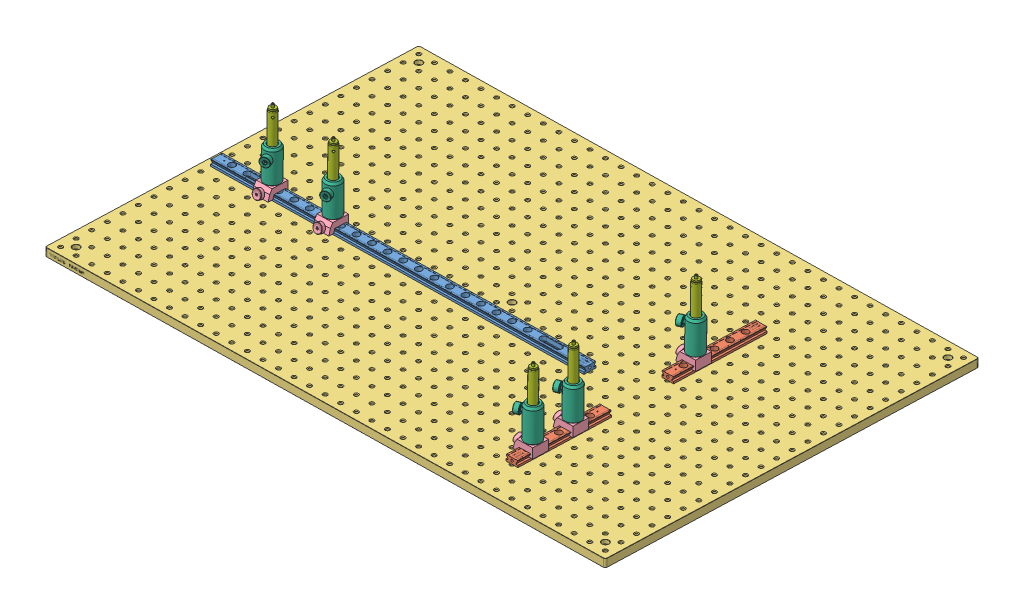
SolidWorks assembly OpenCALAssembly, configuration Default. Lengths in mm.
Overall size (900.56 165.28 600.29).
29 component instances, 7 part files, 30 mates.
Components (placement in the parent):
- RLA600_M-Solidworks-1: RLA600_M-Solidworks [Default] at (212.74 428.5429 890.6377) x (0.000793 -0.03295 -0.999457) z (0.999847 0.01748 0.000217) size (19.05 9.53 600)
- RLA150_M-Solidworks-1: RLA150_M-Solidworks [Default] at (587.7819 430.9791 765.7872) x (0.999847 0.01748 0.000217) z (-0.000793 0.03295 0.999457) size (19.05 9.53 150)
- RLA150_M-Solidworks-2: RLA150_M-Solidworks [Default] at (587.5835 439.2167 1015.6513) x (-0.999847 -0.01748 -0.000217) z (0.000793 -0.03295 -0.999457) size (19.05 9.53 150)
- MB6090_M-Solidworks-1: MB6090_M-Solidworks [Default] at (350.5593 411.9431 853.774) x (0.999847 0.01748 0.000217) z (-0.000793 0.03295 0.999457) size (900 12.7 600)
- Rail-Post^OpenCALAssembly-1: Rail-Post^OpenCALAssembly [Default] at (243.8757 -121.8493 -138.0671) x (0.999969 -0.007878 0.000659) z (-0.000645 0.001893 0.999998) size (37.63 121.62 44.58) (virtual)
  - RC1-Solidworks-1: RC1-Solidworks [Default] at (-258.0543 541.4605 1048.8284) x (0.999678 0.025357 -0.000394) z (-0.000279 0.026514 0.999648) size (25.4 16.53 39.23)
  - socket head cap screw_am-1: socket head cap screw_am [B18.3.1M - 6 x 1.0 x 10 Hex SHCS -- 10NHX] at (-245.5045 547.2464 1029.7741) x (-0.025359 0.999327 -0.026513) z (0.026513 0.027184 0.999279) size (16 10 10)
  - PH50_M-Solidworks-1: PH50_M-Solidworks [Default] at (-244.0284 576.1062 1033.7923) x (0.926646 0.013547 -0.375692) z (0.37508 0.034095 0.926365) size (25 50.44 35.14)
  - TR75_M-Solidworks-1: TR75_M-Solidworks [Default] at (-246.3606 580.9852 1028.879) x (0.691707 -0.001607 -0.722176) z (0.721732 0.036653 0.691201) size (12.67 80.02 12.87)
- Rail-Post^OpenCALAssembly-2: Rail-Post^OpenCALAssembly [Default] at (341.3904 -120.1445 -138.0459) x (0.999969 -0.007878 0.000659) z (-0.000645 0.001893 0.999998) size (37.63 121.62 44.58) (virtual)
  - RC1-Solidworks-1: RC1-Solidworks [Default] at (-258.0543 541.4605 1048.8284) x (0.999678 0.025357 -0.000394) z (-0.000279 0.026514 0.999648) size (25.4 16.53 39.23)
  - socket head cap screw_am-1: socket head cap screw_am [B18.3.1M - 6 x 1.0 x 10 Hex SHCS -- 10NHX] at (-245.5045 547.2464 1029.7741) x (-0.025359 0.999327 -0.026513) z (0.026513 0.027184 0.999279) size (16 10 10)
  - PH50_M-Solidworks-1: PH50_M-Solidworks [Default] at (-244.0284 576.1062 1033.7923) x (0.926646 0.013547 -0.375692) z (0.37508 0.034095 0.926365) size (25 50.44 35.14)
  - TR75_M-Solidworks-1: TR75_M-Solidworks [Default] at (-246.3606 580.9852 1028.879) x (0.691707 -0.001607 -0.722176) z (0.721732 0.036653 0.691201) size (12.67 80.02 12.87)
- Rail-Post^OpenCALAssembly-4: Rail-Post^OpenCALAssembly [Default] at (1642.5862 -51.8881 1242.018) x (0.000044 0.007607 0.999971) z (-0.998822 -0.048519 0.000413) size (37.63 121.62 44.58) (virtual)
  - RC1-Solidworks-1: RC1-Solidworks [Default] at (-258.0543 541.4605 1048.8284) x (0.999678 0.025357 -0.000394) z (-0.000279 0.026514 0.999648) size (25.4 16.53 39.23)
  - socket head cap screw_am-1: socket head cap screw_am [B18.3.1M - 6 x 1.0 x 10 Hex SHCS -- 10NHX] at (-245.5045 547.2464 1029.7741) x (-0.025359 0.999327 -0.026513) z (0.026513 0.027184 0.999279) size (16 10 10)
  - PH50_M-Solidworks-1: PH50_M-Solidworks [Default] at (-244.0284 576.1062 1033.7923) x (0.926646 0.013547 -0.375692) z (0.37508 0.034095 0.926365) size (25 50.44 35.14)
  - TR75_M-Solidworks-1: TR75_M-Solidworks [Default] at (-246.3606 580.9852 1028.879) x (0.691707 -0.001607 -0.722176) z (0.721732 0.036653 0.691201) size (12.67 80.02 12.87)
- Rail-Post^OpenCALAssembly-6: Rail-Post^OpenCALAssembly [Default] at (1642.7424 -58.374 1045.2874) x (0.000044 0.007607 0.999971) z (-0.998822 -0.048519 0.000413) size (37.63 121.62 44.58) (virtual)
  - RC1-Solidworks-1: RC1-Solidworks [Default] at (-258.0543 541.4605 1048.8284) x (0.999678 0.025357 -0.000394) z (-0.000279 0.026514 0.999648) size (25.4 16.53 39.23)
  - socket head cap screw_am-1: socket head cap screw_am [B18.3.1M - 6 x 1.0 x 10 Hex SHCS -- 10NHX] at (-245.5045 547.2464 1029.7741) x (-0.025359 0.999327 -0.026513) z (0.026513 0.027184 0.999279) size (16 10 10)
  - PH50_M-Solidworks-1: PH50_M-Solidworks [Default] at (-244.0284 576.1062 1033.7923) x (0.926646 0.013547 -0.375692) z (0.37508 0.034095 0.926365) size (25 50.44 35.14)
  - TR75_M-Solidworks-1: TR75_M-Solidworks [Default] at (-246.3606 580.9852 1028.879) x (0.691707 -0.001607 -0.722176) z (0.721732 0.036653 0.691201) size (12.67 80.02 12.87)
- Rail-Post^OpenCALAssembly-8: Rail-Post^OpenCALAssembly [Default] at (1642.581 -49.6743 1306.6232) x (0.000044 0.007607 0.999971) z (-0.998822 -0.048519 0.000413) size (37.63 121.62 44.58) (virtual)
  - RC1-Solidworks-1: RC1-Solidworks [Default] at (-258.0543 541.4605 1048.8284) x (0.999678 0.025357 -0.000394) z (-0.000279 0.026514 0.999648) size (25.4 16.53 39.23)
  - socket head cap screw_am-1: socket head cap screw_am [B18.3.1M - 6 x 1.0 x 10 Hex SHCS -- 10NHX] at (-245.5045 547.2464 1029.7741) x (-0.025359 0.999327 -0.026513) z (0.026513 0.027184 0.999279) size (16 10 10)
  - PH50_M-Solidworks-1: PH50_M-Solidworks [Default] at (-244.0284 576.1062 1033.7923) x (0.926646 0.013547 -0.375692) z (0.37508 0.034095 0.926365) size (25 50.44 35.14)
  - TR75_M-Solidworks-1: TR75_M-Solidworks [Default] at (-246.3606 580.9852 1028.879) x (0.691707 -0.001607 -0.722176) z (0.721732 0.036653 0.691201) size (12.67 80.02 12.87)
Mates (geometry in assembly coordinates):
- Concentric5: concentric aligned: cylinder of RLA600_M-Solidworks-1 through (-62.2911 427.9239 890.4398) axis (-0.017463 0.999304 -0.032959) radius 3.3655; circle of MB6090_M-Solidworks-1
- Concentric6: concentric aligned: cylinder of RLA600_M-Solidworks-1 through (487.6248 437.538 890.5594) axis (-0.017463 0.999304 -0.032959) radius 3.3655; circle of MB6090_M-Solidworks-1
- Coincident8: coincident anti-aligned: plane of RLA600_M-Solidworks-1 through (512.7753 429.0243 900.3902) normal (0.017463 -0.999304 0.032959); plane of MB6090_M-Solidworks-1 through (-96.8299 426.6069 1150.0969) normal (-0.017463 0.999304 -0.032959)
- Coincident9: coincident anti-aligned: plane of RLA150_M-Solidworks-2 through (578.2082 431.5024 940.8575) normal (0.017463 -0.999304 0.032959); plane of MB6090_M-Solidworks-1 through (-96.8299 426.6069 1150.0969) normal (-0.017463 0.999304 -0.032959)
- Coincident10: coincident anti-aligned: plane of RLA150_M-Solidworks-1 through (597.3346 428.5404 840.9159) normal (0.017463 -0.999304 0.032959); plane of MB6090_M-Solidworks-1 through (-96.8299 426.6069 1150.0969) normal (-0.017463 0.999304 -0.032959)
- Concentric7: concentric aligned: cylinder of RLA600_M-Solidworks-1 through (-12.2988 428.7979 890.4507) axis (-0.017463 0.999304 -0.032959) radius 5.1562; cylinder of socket head cap screw_am-2 through (-200.2466 470.3352 1027.7075) axis (-0.025357 0.999196 -0.031056) radius 5
- Parallel5: parallel aligned: plane of RLA600_M-Solidworks-1 through (-87.2867 427.5323 884.1048) normal (-0.999847 -0.01748 -0.000217); plane of Rail-Post^OpenCALAssembly-1/RC1-Solidworks-1 through (-10.5574 422.7142 877.982) normal (-0.999847 -0.01748 -0.000217)
- Coincident23: coincident anti-aligned: plane of RLA600_M-Solidworks-1 through (512.6371 437.1668 881.4679) normal (0.009352 -0.524324 -0.851468); plane of Rail-Post^OpenCALAssembly-1/RC1-Solidworks-1 through (14.7938 425.6602 883.0857) normal (-0.009352 0.524324 0.851468)
- Parallel6: parallel aligned: plane of RLA600_M-Solidworks-1 through (-87.2867 427.5323 884.1048) normal (-0.999847 -0.01748 -0.000217); plane of Rail-Post^OpenCALAssembly-1/RC1-Solidworks-1 through (-10.5574 422.7142 877.982) normal (-0.999847 -0.01748 -0.000217)
- Coincident24: coincident: line of RLA600_M-Solidworks-1 through (512.6238 437.9283 881.4428) axis (-0.999847 -0.01748 -0.000217); plane of Rail-Post^OpenCALAssembly-1/RC1-Solidworks-1 through (14.7185 429.7567 900.0847) normal (0.017467 -0.999444 0.028416)
- Parallel7: parallel aligned: plane of RLA600_M-Solidworks-1 through (-87.2867 427.5323 884.1048) normal (-0.999847 -0.01748 -0.000217); plane of Rail-Post^OpenCALAssembly-2/RC1-Solidworks-1 through (86.9572 424.419 878.0032) normal (-0.999847 -0.01748 -0.000217)
- Coincident25: coincident anti-aligned: plane of RLA600_M-Solidworks-1 through (512.6371 437.1668 881.4679) normal (0.009352 -0.524324 -0.851468); plane of Rail-Post^OpenCALAssembly-2/RC1-Solidworks-1 through (112.3085 427.365 883.1069) normal (-0.009352 0.524324 0.851468)
- Parallel8: parallel aligned: plane of RLA600_M-Solidworks-1 through (-87.2867 427.5323 884.1048) normal (-0.999847 -0.01748 -0.000217); plane of Rail-Post^OpenCALAssembly-2/RC1-Solidworks-1 through (86.9572 424.419 878.0032) normal (-0.999847 -0.01748 -0.000217)
- Coincident26: coincident: line of RLA600_M-Solidworks-1 through (512.6238 437.9283 881.4428) axis (-0.999847 -0.01748 -0.000217); plane of Rail-Post^OpenCALAssembly-2/RC1-Solidworks-1 through (112.2332 431.4615 900.1059) normal (0.017467 -0.999444 0.028416)
- Parallel11: parallel aligned: plane of RLA150_M-Solidworks-2 through (581.2418 441.0767 940.5442) normal (0.000793 -0.03295 -0.999457); plane of Rail-Post^OpenCALAssembly-4/RC1-Solidworks-1 through (600.2998 436.7637 980.2933) normal (0.000793 -0.03295 -0.999457)
- Coincident29: coincident anti-aligned: plane of RLA150_M-Solidworks-2 through (596.6959 440.5852 940.5727) normal (0.876819 -0.480535 0.016538); plane of Rail-Post^OpenCALAssembly-4/RC1-Solidworks-1 through (595.0618 439.8415 1005.6015) normal (-0.876819 0.480535 -0.016538)
- Parallel12: parallel aligned: plane of RLA150_M-Solidworks-2 through (581.2418 441.0767 940.5442) normal (0.000793 -0.03295 -0.999457); plane of Rail-Post^OpenCALAssembly-4/RC1-Solidworks-1 through (600.2998 436.7637 980.2933) normal (0.000793 -0.03295 -0.999457)
- Coincident30: coincident: line of RLA150_M-Solidworks-2 through (596.6826 441.3467 940.5476) axis (-0.000793 0.03295 0.999457); plane of Rail-Post^OpenCALAssembly-4/RC1-Solidworks-1 through (577.8779 443.0744 1005.4813) normal (0.022008 -0.999214 0.03296)
- Concentric13: concentric anti-aligned: cylinder of RLA150_M-Solidworks-2 through (587.55 441.7572 965.5404) axis (-0.017463 0.999304 -0.032959) radius 5.1562; cone of MB6090_M-Solidworks-1 through (587.7119 432.4927 965.8459) axis (0.017463 -0.999304 0.032959)
- Concentric14: concentric anti-aligned: cylinder of RLA150_M-Solidworks-2 through (587.4707 445.0522 1065.4861) axis (-0.017463 0.999304 -0.032959) radius 5.1562; cone of MB6090_M-Solidworks-1 through (587.6326 435.7877 1065.7916) axis (0.017463 -0.999304 0.032959)
- Concentric15: concentric anti-aligned: cylinder of RLA150_M-Solidworks-1 through (587.669 436.8147 815.6219) axis (-0.017463 0.999304 -0.032959) radius 3.3655; cone of MB6090_M-Solidworks-1 through (587.8309 427.5501 815.9274) axis (0.017463 -0.999304 0.032959)
- Concentric16: concentric anti-aligned: cylinder of RLA150_M-Solidworks-1 through (587.7484 433.5197 715.6762) axis (-0.017463 0.999304 -0.032959) radius 5.1562; cone of MB6090_M-Solidworks-1 through (587.9103 424.2551 715.9818) axis (0.017463 -0.999304 0.032959)
- Parallel13: parallel aligned: plane of RLA150_M-Solidworks-2 through (581.2418 441.0767 940.5442) normal (0.000793 -0.03295 -0.999457); plane of Rail-Post^OpenCALAssembly-6/RC1-Solidworks-1 through (600.456 430.2779 783.5628) normal (0.000793 -0.03295 -0.999457)
- Coincident31: coincident anti-aligned: plane of RLA150_M-Solidworks-2 through (596.6959 440.5852 940.5727) normal (0.876819 -0.480535 0.016538); plane of Rail-Post^OpenCALAssembly-6/RC1-Solidworks-1 through (595.218 433.3557 808.8709) normal (-0.876819 0.480535 -0.016538)
- Parallel14: parallel aligned: plane of RLA150_M-Solidworks-2 through (581.2418 441.0767 940.5442) normal (0.000793 -0.03295 -0.999457); plane of Rail-Post^OpenCALAssembly-6/RC1-Solidworks-1 through (600.456 430.2779 783.5628) normal (0.000793 -0.03295 -0.999457)
- Coincident32: coincident: line of RLA150_M-Solidworks-2 through (596.6826 441.3467 940.5476) axis (-0.000793 0.03295 0.999457); plane of Rail-Post^OpenCALAssembly-6/RC1-Solidworks-1 through (578.0341 436.5886 808.7507) normal (0.022008 -0.999214 0.03296)
- Parallel17: parallel anti-aligned: plane of RLA150_M-Solidworks-1 through (593.9684 438.0028 840.6013) normal (-0.000793 0.03295 0.999457); plane of Rail-Post^OpenCALAssembly-8/RC1-Solidworks-1 through (600.2946 438.9776 1044.8985) normal (0.000793 -0.03295 -0.999457)
- Coincident35: coincident anti-aligned: plane of RLA150_M-Solidworks-1 through (596.7753 437.2902 840.627) normal (0.876819 -0.480535 0.016538); plane of Rail-Post^OpenCALAssembly-8/RC1-Solidworks-1 through (595.0565 442.0554 1070.2067) normal (-0.876819 0.480535 -0.016538)
- Parallel18: parallel aligned: plane of RLA150_M-Solidworks-1 through (594.0874 433.0603 690.6828) normal (0.000793 -0.03295 -0.999457); plane of Rail-Post^OpenCALAssembly-8/RC1-Solidworks-1 through (600.2946 438.9776 1044.8985) normal (0.000793 -0.03295 -0.999457)
- Coincident36: coincident: line of RLA150_M-Solidworks-1 through (578.5276 437.7329 840.5979) axis (0.000793 -0.03295 -0.999457); plane of Rail-Post^OpenCALAssembly-8/RC1-Solidworks-1 through (577.8727 445.2883 1070.0864) normal (0.022008 -0.999214 0.03296)
